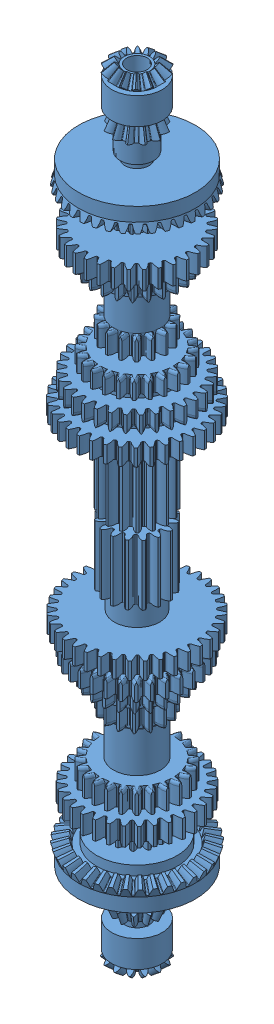
SolidWorks assembly 电机齿轮打印, configuration 默认. Lengths in mm.
Overall size (19 116.8 19).
24 component instances, 8 part files, 45 mates.
Components (placement in the parent):
- 齿轮32x24-1: 齿轮32x24 [默认] at (-14.4241 -2.2842 27.3648) x (-0.082432 0 -0.996597) z (0 -1 0) size (16.99 16.99 14.75) (hidden)
- 齿轮24x32-1: 齿轮24x32 [默认] at (-17.2089 -18.3169 27.8601) x (0.715914 0 -0.698188) z (0 1 0) size (17.17 17.17 5.51) (hidden)
- 36锥齿轮零件-1: 36锥齿轮零件 [默认] at (-16.6413 -29.4199 29.1548) x (0 -1 0) z (0.790717 0 0.612182) size (7.28 18.19 18.19) (hidden)
- 电机输出小齿轮12X2-1: 电机输出小齿轮12X2 [GB - Straight bevel pinion 0.5M12PT 36GT 20PA 2FW ---12O5H12MD2.0N] at (-16.6413 -33.5043 29.1548) x (0 -1 0) z (0.808929 0 0.587906) size (5.09 6.91 6.91) (hidden)
- 装配体齿轮连接件-1: 装配体齿轮连接件 [默认] at (-16.6413 -21.3741 29.1548) x (0.973829 0 0.227281) z (0 -1 0) size (3.6 3.6 1) (hidden)
- 装配体齿轮连接件-2: 装配体齿轮连接件 [默认] at (-16.6413 -5.6241 29.1548) x (0.194178 0 -0.980966) z (0 -1 0) size (3.6 3.6 1) (hidden)
- 装配体齿轮连接件-3: 装配体齿轮连接件 [默认] at (-16.6413 38.3759 29.1548) x (0.824007 0 0.56658) z (0 -1 0) size (3.6 3.6 1) (hidden)
- 装配体齿轮连接件-4: 装配体齿轮连接件 [默认] at (-16.6413 -29.6585 29.1548) x (0.523547 0 0.851997) z (0 -1 0) size (3.6 3.6 1) (hidden)
- 装配体齿轮连接件-5: 装配体齿轮连接件 [默认] at (-16.6413 -35.4342 29.1548) x (0.941815 0 0.336133) z (0 -1 0) size (3.6 3.6 1) (hidden)
- 前后传动锥齿-1: 前后传动锥齿 [GB - Straight miter gear 0.5M14T 20PA 2FW ---14O7H6MD3.0N] at (-16.6413 -40.4342 29.1548) x (0 -1 0) z (-0.322036 0 0.946727) size (6.09 7.64 7.8) (hidden)
- 前后传动锥齿-2: 前后传动锥齿 [GB - Straight miter gear 0.5M14T 20PA 2FW ---14O7H6MD3.0N] at (-16.6413 72.1859 29.1548) x (0 1 0) z (-0.551252 0 0.834339) size (6.09 7.64 7.8) (hidden)
- 装配体齿轮连接件-6: 装配体齿轮连接件 [默认] at (-16.6413 67.1859 29.1548) x (-0.842475 0 -0.538736) z (0 1 0) size (3.6 3.6 1) (hidden)
- 装配体齿轮连接件-7: 装配体齿轮连接件 [默认] at (-16.6413 61.4102 29.1548) x (-0.994169 0 0.107833) z (0 1 0) size (3.6 3.6 1) (hidden)
- 装配体齿轮连接件-8: 装配体齿轮连接件 [默认] at (-16.6413 30.8759 29.1548) x (-0.952518 0 -0.304482) z (0 1 0) size (3.6 3.6 1) (hidden)
- 装配体齿轮连接件-9: 装配体齿轮连接件 [默认] at (-16.6413 53.1259 29.1548) x (-0.90003 0 0.435828) z (0 1 0) size (3.6 3.6 1) (hidden)
- 电机输出小齿轮12X2-2: 电机输出小齿轮12X2 [GB - Straight bevel pinion 0.5M12PT 36GT 20PA 2FW ---12O5H12MD2.0N] at (-16.6413 65.256 29.1548) x (0 1 0) z (-0.960145 0 -0.279503) size (5.09 6.91 6.91) (hidden)
- 齿轮24x32-2: 齿轮24x32 [默认] at (-15.2281 50.0686 29.1194) x (0.328431 0 -0.944528) z (0 -1 0) size (17.17 17.17 5.51) (hidden)
- 齿轮32x24-2: 齿轮32x24 [默认] at (-13.7931 34.036 29.0647) x (0.587759 0 0.809036) z (0 1 0) size (16.99 16.99 14.75) (hidden)
- 36锥齿轮零件-2: 36锥齿轮零件 [默认] at (-16.6413 61.1716 29.1548) x (0 1 0) z (0.164736 0 -0.986338) size (7.28 18.19 18.19) (hidden)
- 电机传动3mm-1: 电机传动3mm [默认] at (-13.5899 47.6214 30.0256) x (0.987621 0 0.15686) z (0 -1 0) size (18.99 18.99 14.5) (hidden)
- 电机传动3mm-2: 电机传动3mm [默认] at (-15.5869 -15.8697 26.1619) x (0.44323 0 -0.896408) z (0 1 0) size (18.99 18.99 14.5) (hidden)
- 装配体齿轮连接件-12: 装配体齿轮连接件 [默认] at (-16.6413 0.8759 29.1548) x (0.194178 0 -0.980966) z (0 -1 0) size (3.6 3.6 1) (hidden)
- 装配体齿轮连接件-13: 装配体齿轮连接件 [默认] at (-16.6413 16.3759 29.1548) x (0.194178 0 -0.980966) z (0 -1 0) size (3.6 3.6 1) (hidden)
- 齿轮整体零件-1: 齿轮整体零件 [默认] at origin size (19 116.8 19)
Mates (geometry in assembly coordinates):
- 同心9: concentric aligned: cylinder of 电机输出小齿轮12X2-1 through (-16.6413 -45.5043 29.1548) axis (0 1 0) radius 1.025; cylinder of 装配体齿轮连接件-4 through (-16.6413 -30.6585 29.1548) axis (0 1 0) radius 1.6
- 重合9: coincident anti-aligned: plane of 电机输出小齿轮12X2-1 through (-16.6413 -30.6585 29.1548) normal (0 1 0); plane of 装配体齿轮连接件-4 through (-16.6413 -30.6585 29.1548) normal (0 -1 0)
- 同心10: concentric aligned: cylinder of 电机输出小齿轮12X2-1 through (-16.6413 -45.5043 29.1548) axis (0 1 0) radius 1.025; cylinder of 装配体齿轮连接件-5 through (-16.6413 -36.4342 29.1548) axis (0 1 0) radius 1.8
- 重合10: coincident anti-aligned: plane of 电机输出小齿轮12X2-1 through (-16.6413 -35.4342 29.1548) normal (0 -1 0); plane of 装配体齿轮连接件-5 through (-16.6413 -35.4342 29.1548) normal (0 1 0)
- 同心11: concentric aligned: cylinder of 装配体齿轮连接件-5 through (-16.6413 -36.4342 29.1548) axis (0 1 0) radius 1.6; cylinder of 前后传动锥齿-1 through (-16.6413 -46.4342 29.1548) axis (0 1 0) radius 1.525
- 重合11: coincident anti-aligned: plane of 装配体齿轮连接件-5 through (-16.6413 -36.4342 29.1548) normal (0 -1 0); plane of 前后传动锥齿-1 through (-16.6413 -36.4342 29.1548) normal (0 1 0)
- 同心16: concentric aligned: cylinder of 装配体齿轮连接件-6 through (-16.6413 68.1859 29.1548) axis (0 -1 0) radius 1.8; cylinder of 电机输出小齿轮12X2-2 through (-16.6413 77.256 29.1548) axis (0 -1 0) radius 1.025
- 同心17: concentric aligned: cylinder of 前后传动锥齿-2 through (-16.6413 78.1859 29.1548) axis (0 -1 0) radius 1.525; cylinder of 装配体齿轮连接件-6 through (-16.6413 68.1859 29.1548) axis (0 -1 0) radius 1.6
- 同心20: concentric aligned: cylinder of 装配体齿轮连接件-7 through (-16.6413 62.4102 29.1548) axis (0 -1 0) radius 1.6; cylinder of 电机输出小齿轮12X2-2 through (-16.6413 77.256 29.1548) axis (0 -1 0) radius 1.025
- 重合13: coincident anti-aligned: plane of 装配体齿轮连接件-6 through (-16.6413 67.1859 29.1548) normal (0 -1 0); plane of 电机输出小齿轮12X2-2 through (-16.6413 67.1859 29.1548) normal (0 1 0)
- 重合14: coincident anti-aligned: plane of 前后传动锥齿-2 through (-16.6413 68.1859 29.1548) normal (0 -1 0); plane of 装配体齿轮连接件-6 through (-16.6413 68.1859 29.1548) normal (0 1 0)
- 重合18: coincident anti-aligned: plane of 装配体齿轮连接件-7 through (-16.6413 62.4102 29.1548) normal (0 1 0); plane of 电机输出小齿轮12X2-2 through (-16.6413 62.4102 29.1548) normal (0 -1 0)
- 同心22: concentric anti-aligned: cylinder of 齿轮32x24-1 through (-16.6413 -9.6231 29.1548) axis (0 -1 0) radius 1.1; cylinder of 装配体齿轮连接件-1 through (-16.6413 -22.3741 29.1548) axis (0 1 0) radius 1.8
- 重合24: coincident anti-aligned: plane of 齿轮32x24-1 through (-16.6413 -21.3741 29.1548) normal (0 -1 0); plane of 装配体齿轮连接件-1 through (-16.6413 -21.3741 29.1548) normal (0 1 0)
- 同心23: concentric anti-aligned: cylinder of 36锥齿轮零件-1 through (-16.6413 -21.6064 29.1548) axis (0 -1 0) radius 1.1; cylinder of 装配体齿轮连接件-4 through (-16.6413 -30.6585 29.1548) axis (0 1 0) radius 1.8
- 重合25: coincident anti-aligned: plane of 36锥齿轮零件-1 through (-16.6413 -29.6585 29.1548) normal (0 -1 0); plane of 装配体齿轮连接件-4 through (-16.6413 -29.6585 29.1548) normal (0 1 0)
- 同心24: concentric anti-aligned: cylinder of 齿轮24x32-1 through (-16.6413 -0.1231 29.1548) axis (0 -1 0) radius 1.525; cylinder of 装配体齿轮连接件-3 through (-16.6413 37.3759 29.1548) axis (0 1 0) radius 1.8
- 重合29: coincident anti-aligned: plane of 齿轮24x32-1 through (-16.6413 -5.6241 29.1548) normal (0 -1 0); plane of 装配体齿轮连接件-2 through (-16.6413 -5.6241 29.1548) normal (0 1 0)
- 同心26: concentric anti-aligned: cylinder of 齿轮24x32-1 through (-16.6413 -0.1231 29.1548) axis (0 -1 0) radius 1.525; cylinder of 装配体齿轮连接件-2 through (-16.6413 -6.6241 29.1548) axis (0 1 0) radius 1.6
- 同心27: concentric anti-aligned: cylinder of 36锥齿轮零件-1 through (-16.6413 -21.6064 29.1548) axis (0 -1 0) radius 1.1; cylinder of 装配体齿轮连接件-1 through (-16.6413 -22.3741 29.1548) axis (0 1 0) radius 1.8
- 重合30: coincident anti-aligned: plane of 齿轮32x24-1 through (-16.6413 -6.6241 29.1548) normal (0 1 0); plane of 装配体齿轮连接件-2 through (-16.6413 -6.6241 29.1548) normal (0 -1 0)
- 重合31: coincident anti-aligned: plane of 36锥齿轮零件-1 through (-16.6413 -22.3741 29.1548) normal (0 1 0); plane of 装配体齿轮连接件-1 through (-16.6413 -22.3741 29.1548) normal (0 -1 0)
- 同心29: concentric anti-aligned: cylinder of 齿轮32x24-1 through (-16.6413 -9.6231 29.1548) axis (0 -1 0) radius 1.1; cylinder of 装配体齿轮连接件-2 through (-16.6413 -6.6241 29.1548) axis (0 1 0) radius 1.8
- 同心30: concentric aligned: cylinder of 齿轮24x32-1 through (-16.6413 -0.1231 29.1548) axis (0 -1 0) radius 1.525; cylinder of 装配体齿轮连接件-8 through (-16.6413 31.8759 29.1548) axis (0 -1 0) radius 1.8
- 重合34: coincident anti-aligned: plane of 装配体齿轮连接件-8 through (-16.6413 31.8759 29.1548) normal (0 1 0); plane of 齿轮24x32-2 through (-16.6413 31.8759 29.1548) normal (0 -1 0)
- 同心31: concentric anti-aligned: cylinder of 装配体齿轮连接件-8 through (-16.6413 31.8759 29.1548) axis (0 -1 0) radius 1.8; cylinder of 齿轮24x32-2 through (-16.6413 31.8749 29.1548) axis (0 1 0) radius 1.525
- 同心32: concentric aligned: cylinder of 装配体齿轮连接件-3 through (-16.6413 37.3759 29.1548) axis (0 1 0) radius 1.8; cylinder of 齿轮24x32-2 through (-16.6413 31.8749 29.1548) axis (0 1 0) radius 1.525
- 重合35: coincident anti-aligned: plane of 装配体齿轮连接件-3 through (-16.6413 37.3759 29.1548) normal (0 -1 0); plane of 齿轮24x32-2 through (-16.6413 37.3759 29.1548) normal (0 1 0)
- 重合36: coincident anti-aligned: plane of 装配体齿轮连接件-3 through (-16.6413 38.3759 29.1548) normal (0 1 0); plane of 齿轮32x24-2 through (-16.6413 38.3759 29.1548) normal (0 -1 0)
- 同心33: concentric aligned: cylinder of 装配体齿轮连接件-3 through (-16.6413 37.3759 29.1548) axis (0 1 0) radius 1.8; cylinder of 齿轮32x24-2 through (-16.6413 41.3759 29.1548) axis (0 1 0) radius 3.5
- 重合37: coincident anti-aligned: plane of 装配体齿轮连接件-9 through (-16.6413 53.1259 29.1548) normal (0 -1 0); plane of 齿轮32x24-2 through (-16.6413 53.1259 29.1548) normal (0 1 0)
- 同心34: concentric anti-aligned: cylinder of 装配体齿轮连接件-9 through (-16.6413 54.1259 29.1548) axis (0 -1 0) radius 1.8; cylinder of 齿轮32x24-2 through (-16.6413 41.3749 29.1548) axis (0 1 0) radius 1.1
- 同心35: concentric anti-aligned: cylinder of 装配体齿轮连接件-9 through (-16.6413 54.1259 29.1548) axis (0 -1 0) radius 1.6; cylinder of 36锥齿轮零件-2 through (-16.6413 53.3581 29.1548) axis (0 1 0) radius 1.1
- 重合38: coincident anti-aligned: plane of 装配体齿轮连接件-9 through (-16.6413 54.1259 29.1548) normal (0 1 0); plane of 36锥齿轮零件-2 through (-16.6413 54.1259 29.1548) normal (0 -1 0)
- 同心36: concentric anti-aligned: cylinder of 装配体齿轮连接件-7 through (-16.6413 62.4102 29.1548) axis (0 -1 0) radius 1.8; cylinder of 36锥齿轮零件-2 through (-16.6413 53.3581 29.1548) axis (0 1 0) radius 1.1
- 重合39: coincident anti-aligned: plane of 装配体齿轮连接件-7 through (-16.6413 61.4102 29.1548) normal (0 -1 0); plane of 36锥齿轮零件-2 through (-16.6413 61.4102 29.1548) normal (0 1 0)
- 同心37: concentric aligned: cylinder of 装配体齿轮连接件-8 through (-16.6413 31.8759 29.1548) axis (0 -1 0) radius 1.8; cylinder of 电机传动3mm-1 through (-16.6413 30.8769 29.1548) axis (0 -1 0) radius 1.6
- 重合40: coincident anti-aligned: plane of 装配体齿轮连接件-8 through (-16.6413 30.8759 29.1548) normal (0 -1 0); plane of 电机传动3mm-1 through (-16.6413 30.8759 29.1548) normal (0 1 0)
- 同心38: concentric aligned: cylinder of 电机传动3mm-2 through (-16.6413 0.8749 29.1548) axis (0 1 0) radius 1.6; cylinder of 装配体齿轮连接件-12 through (-16.6413 -0.1241 29.1548) axis (0 1 0) radius 1.8
- 同心39: concentric anti-aligned: cylinder of 电机传动3mm-1 through (-16.6413 30.8769 29.1548) axis (0 -1 0) radius 1.6; cylinder of 装配体齿轮连接件-13 through (-16.6413 15.3759 29.1548) axis (0 1 0) radius 1.8
- 同心40: concentric aligned: cylinder of 电机传动3mm-2 through (-16.6413 0.8749 29.1548) axis (0 1 0) radius 1.6; cylinder of 装配体齿轮连接件-13 through (-16.6413 15.3759 29.1548) axis (0 1 0) radius 1.8
- 重合41: coincident anti-aligned: plane of 电机传动3mm-1 through (-16.6413 16.3759 29.1548) normal (0 -1 0); plane of 装配体齿轮连接件-13 through (-16.6413 16.3759 29.1548) normal (0 1 0)
- 重合42: coincident anti-aligned: plane of 电机传动3mm-2 through (-16.6413 15.3759 29.1548) normal (0 1 0); plane of 装配体齿轮连接件-13 through (-16.6413 15.3759 29.1548) normal (0 -1 0)
- 重合43: coincident anti-aligned: plane of 电机传动3mm-2 through (-16.6413 0.8759 29.1548) normal (0 -1 0); plane of 装配体齿轮连接件-12 through (-16.6413 0.8759 29.1548) normal (0 1 0)
- 重合44: coincident anti-aligned: plane of 齿轮24x32-1 through (-16.6413 -0.1241 29.1548) normal (0 1 0); plane of 装配体齿轮连接件-12 through (-16.6413 -0.1241 29.1548) normal (0 -1 0)
